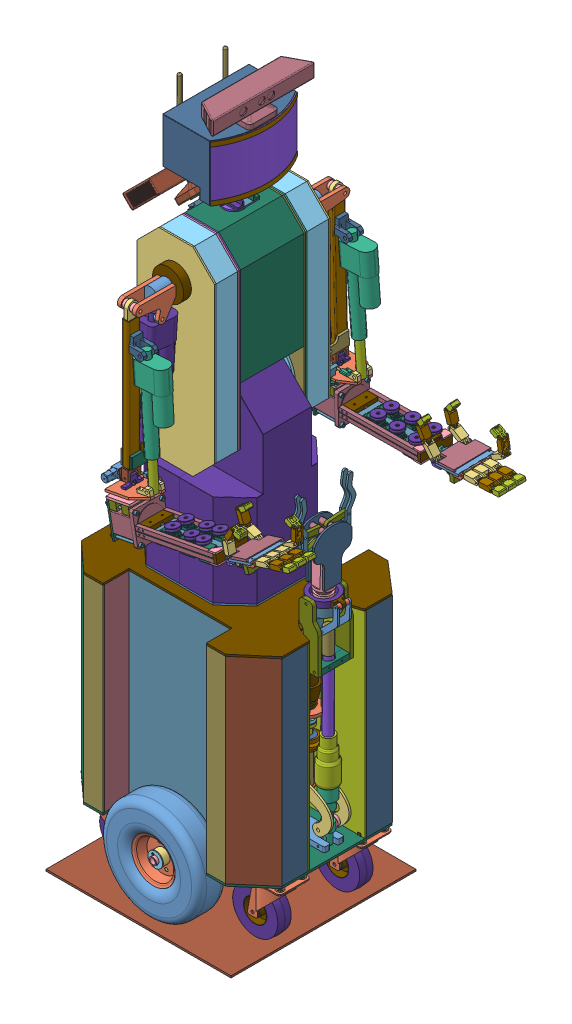
SolidWorks assembly sorbot, configuration По умолчанию. Lengths in mm. (continued)
Mates (geometry in assembly coordinates): (continued)
- Совпадение121: coincident anti-aligned: plane of bottom-2 through (-49.3372 51.9368 -286.1821) normal (0 1 0); plane of wall6-1 through (263.1742 51.9368 -58.2424) normal (0 -1 0)
- Совпадение122: coincident aligned: line of bottom-2 through (267.1742 51.9368 11.9714) axis (0 0 -1); line of wall6-1 through (267.1742 51.9368 11.8264) axis (0 0 -1)
- Параллельность26: parallel aligned: line of bottom-2 through (184.9009 51.9368 82.4522) axis (0.759435 0 -0.650583); line of wall7-1 through (184.8921 51.9368 82.4377) axis (0.759435 0 -0.650583)
- Совпадение127: coincident anti-aligned: plane of bottom-2 through (-49.3372 51.9368 -286.1821) normal (0 1 0); plane of wall7-1 through (263.5537 51.9368 9.7838) normal (0 -1 0)
- Совпадение131: coincident anti-aligned: line of bottom-2 through (267.1742 51.9368 11.9714) axis (0 0 -1); line of wall6-3 through (267.1742 51.9368 -286.3112) axis (0 0 1)
- Совпадение132: coincident anti-aligned: line of wall6-3 through (267.1742 51.9368 -216.2424) axis (0 1 0); line of wall2-2 through (267.1741 585.1505 -216.2424) axis (0 -1 0)
- Совпадение136: coincident aligned: line of bottom-2 through (132.9009 51.9368 12.4522) axis (0 0 1); line of wall8-1 through (132.9009 51.9368 78.4522) axis (0 0 1)
- Совпадение137: coincident aligned: line of bottom-2 through (132.9009 51.9368 82.4522) axis (1 0 0); line of wall8-1 through (132.9009 51.9368 82.4522) axis (1 0 0)
- Совпадение142: coincident anti-aligned: plane of bottom-2 through (-49.3372 51.9368 -286.1821) normal (0 1 0); plane of wall8-2 through (141.3107 51.9368 -178.9033) normal (0 -1 0)
- Совпадение143: coincident anti-aligned: plane of wall8-1 through (132.9009 637.4067 78.4522) normal (0 0 -1); plane of wall9-1 through (132.9009 655.1671 78.4522) normal (0 0 1)
- Совпадение144: coincident anti-aligned: plane of bottom-2 through (-49.3372 51.9368 -286.1821) normal (0 1 0); plane of wall9-1 through (132.9009 51.9368 78.4522) normal (0 -1 0)
- Совпадение145: coincident aligned: line of bottom-2 through (132.9009 51.9368 12.4522) axis (0 0 1); line of wall9-1 through (132.9009 51.9368 8.55) axis (0 0 1)
- Совпадение146: coincident aligned: line of bottom-2 through (39.4201 51.9368 12.4522) axis (1 0 0); line of wall10-1 through (-146.6756 51.9368 12.4522) axis (1 0 0)
- Совпадение147: coincident anti-aligned: plane of wall9-1 through (132.9009 655.1671 8.55) normal (-1 0 0); plane of wall10-1 through (132.9009 864.7556 8.4522) normal (1 0 0)
- Совпадение149: coincident anti-aligned: plane of bottom-2 through (-49.3372 51.9368 -286.1821) normal (0 1 0); plane of wall9-2 through (-150.6756 51.9368 78.5322) normal (0 -1 0)
- Совпадение157: coincident anti-aligned: line of wall3-1 through (107.1741 166.4368 -62.2424) axis (0 0 -1); line of wall4-1 through (107.1741 166.4368 -216.2424) axis (0 0 1)
- Совпадение161: coincident anti-aligned: line of wall2-2 through (21.1889 166.4368 -212.2424) axis (1 0 0); line of wall3-1 through (107.1741 166.4368 -212.2424) axis (-1 0 0)
- Совпадение162: coincident anti-aligned: line of wall2-1 through (107.1741 166.4368 -62.2424) axis (-1 0 0); line of wall3-1 through (26.1889 166.4368 -62.2424) axis (1 0 0)
- Совпадение170: coincident anti-aligned: plane of bottom-2 through (-49.3372 51.9368 -286.1821) normal (0 1 0); plane of wall7-v1-1 through (-149.98 51.9368 -93.7194) normal (0 -1 0)
- Параллельность29: parallel anti-aligned: line of bottom-2 through (-275.9596 51.9368 11.9714) axis (0.73854 0 0.67421); line of wall7-v1-1 through (-199.0366 51.9368 82.0998) axis (-0.73854 0 -0.67421)
- Совпадение174: coincident anti-aligned: line of wall7-v1-1 through (-275.9003 51.9368 11.9312) axis (0 1 0); line of wall11-1 through (-275.9003 585.1505 11.9312) axis (0 -1 0)
- Совпадение180: coincident anti-aligned: line of wall7-v1-2 through (-198.8179 51.9368 -356.1236) axis (0 1 0); line of wall8-5 through (-198.8179 585.1505 -356.1236) axis (0 -1 0)
- Совпадение181: coincident anti-aligned: plane of bottom-2 through (-49.3372 51.9368 -286.1821) normal (0 1 0); plane of wall8-5 through (-146.715 51.9368 -356.1236) normal (0 -1 0)
- Параллельность31: parallel aligned: line of bottom-2 through (-146.7539 51.9368 -356.1821) axis (-1 0 0); line of wall8-5 through (-146.715 51.9368 -356.1236) axis (-1 0 0)
- Совпадение182: coincident anti-aligned: plane of bottom-2 through (-49.3372 51.9368 -286.1821) normal (0 1 0); plane of wall9-3 through (-150.8245 51.9368 -282.1286) normal (0 -1 0)
- Совпадение184: coincident anti-aligned: plane of bottom-2 through (-49.3372 51.9368 -286.1821) normal (0 1 0); plane of wall10-v1-1 through (132.7521 51.9368 -286.1286) normal (0 -1 0)
- Совпадение187: coincident aligned: line of wall9-3 through (-146.8245 585.1505 -282.1286) axis (0 -1 0); line of wall10-v1-1 through (-146.8245 585.1505 -282.1286) axis (0 -1 0)
- Совпадение188: coincident anti-aligned: plane of bottom-2 through (-49.3372 51.9368 -286.1821) normal (0 1 0); plane of wall9-4 through (132.7521 51.9368 -282.1286) normal (0 -1 0)
- Совпадение189: coincident aligned: line of wall10-v1-1 through (132.7521 585.1505 -282.1286) axis (0 -1 0); line of wall9-4 through (132.7521 585.1505 -282.1286) axis (0 -1 0)
- Совпадение191: coincident anti-aligned: line of bottom-2 through (184.9009 51.9368 -356.1821) axis (-1 0 0); line of wall8-2 through (132.798 51.9368 -356.1821) axis (1 0 0)
- Совпадение201: coincident anti-aligned: plane of bottom-2 through (-49.3372 51.9368 -286.1821) normal (0 1 0); plane of wall7-3 through (183.3311 51.9368 -352.2595) normal (0 -1 0)
- Параллельность33: parallel aligned: line of bottom-2 through (267.1742 51.9368 -285.7013) axis (-0.759435 0 -0.650583); line of wall7-3 through (267.1973 51.9368 -285.6811) axis (-0.759435 0 -0.650583)
- Параллельность52: parallel anti-aligned: plane of gearmotor-3 through (-22.0648 623.1505 -128.1055) normal (-1 0 0); plane of turret-1/turret-p1-1 through (-22.0648 627.1934 -130.2473) normal (1 0 0)
- Концентричный93: concentric aligned: cylinder of gearmotor-3 through (-20.0648 629.1505 -136.9555) axis (0 -1 0) radius 7; cylinder of turret-1/turret-p1-1 through (-20.0648 627.1934 -136.9555) axis (0 -1 0) radius 7
- Концентричный110: concentric anti-aligned: cylinder of bolt1-2 through (172.9115 63.0264 3.3236) axis (0 -1 0) radius 5; cylinder of bolt1.nut-9 through (172.9115 51.9368 3.3236) axis (0 1 0) radius 5
- Концентричный111: concentric anti-aligned: cylinder of turret-1/turret-p1-1 through (-20.0648 603.2934 -136.9555) axis (0 1 0) radius 74; cylinder of turret.table-1 through (-20.0648 612.7934 -136.9555) axis (0 -1 0) radius 35
- Концентричный112: concentric aligned: cylinder of gearmotor-3 through (-20.0648 629.1505 -136.9555) axis (0 -1 0) radius 7; cylinder of turret.center-1 through (-20.0648 622.7934 -136.9555) axis (0 -1 0) radius 7
- Совпадение223: coincident anti-aligned: plane of turret-1/turret-p1-1 through (-20.0648 607.7934 -136.9555) normal (0 1 0); plane of ? through (-20.0648 607.7934 -136.9555) normal (0 -1 0)
- Совпадение230: coincident anti-aligned: plane of gearmotor.fixture.p2-3 through (10.2084 53.4933 -245.0001) normal (0 1 0); plane of wheel.axis.frame.fixture.p2-3 through (-51.698 53.4933 -213.5833) normal (0 -1 0)
- Совпадение236: coincident anti-aligned: plane of bottom-2 through (-49.3372 51.9368 -286.1821) normal (0 1 0); plane of wall-fixture-3-2 through (213.2226 51.9368 -31.5478) normal (0 -1 0)
- Совпадение242: coincident anti-aligned: plane of gearmotor-2 through (-40.8776 119.0545 -28.1692) normal (0 0 1); plane of gearmotor.fixture.p2.1-1 through (2.1309 53.4368 -28.1692) normal (0 0 -1)
- Совпадение246: coincident anti-aligned: plane of bottom-2 through (-49.3372 51.9368 -286.1821) normal (0 1 0); plane of wheel.axis.frame.fixture.p2-1 through (43.2929 51.9368 -36.1421) normal (0 -1 0)
- Совпадение248: coincident anti-aligned: plane of wheel.axis.frame-4 through (15.3082 32.4368 -66.3906) normal (0 -1 0); plane of wheel.axis.frame.fixture.p1-1 through (42.6901 32.4368 -36.0198) normal (0 1 0)
- Концентричный116: concentric aligned: circle of wheel.axis.frame.fixture.p1-1; circle of wheel.axis.frame.fixture.p2-1
- Совпадение252: coincident anti-aligned: plane of wall7-v1-1 through (-271.8817 585.1505 10.1837) normal (0 1 0); plane of cap-1 through (216.6954 585.1505 -83.7838) normal (0 -1 0)
- Совпадение253: coincident anti-aligned: plane of cap-1 through (216.6954 590.1505 -83.7838) normal (0 1 0); plane of turret-1/turret-p4-1 through (-19.4709 590.1505 -137.0226) normal (0 -1 0)
- Совпадение254: coincident anti-aligned: plane of turret-1/turret-p1-1 through (-20.0648 607.7934 -136.9555) normal (0 1 0); plane of turret.table-1 through (-20.0648 607.7934 -360.2969) normal (0 -1 0)
- Заблокировать30: lock: unknown of ?; unknown of ?
- Заблокировать31: lock: unknown of ?; unknown of ?
- Заблокировать32: lock: unknown of ?; unknown of ?
- Заблокировать33: lock: unknown of ?; unknown of ?
- Заблокировать34: lock: unknown of ?; unknown of ?
- Заблокировать35: lock: unknown of ?; unknown of ?
- Заблокировать36: lock: unknown of ?; unknown of ?
- Заблокировать37: lock: unknown of ?; unknown of ?
- Заблокировать38: lock: unknown of ?; unknown of ?
- Заблокировать39: lock: unknown of ?; unknown of ?
- Заблокировать40: lock: unknown of ?; unknown of ?
- Заблокировать41: lock: unknown of ?; unknown of ?
- Совпадение276: coincident anti-aligned: plane of bottom-2 through (-49.3372 51.9368 -286.1821) normal (0 1 0); plane of wall-fixture-3-3-1 through (-242.5877 51.9368 -17.2349) normal (0 -1 0)
- Совпадение277: coincident anti-aligned: plane of wall7-v1-1 through (-271.8817 -52.2153 10.1837) normal (0.67421 0 -0.73854); plane of wall-fixture-3-3-1 through (-269.5561 51.9368 12.3067) normal (-0.67421 0 0.73854)
- Заблокировать42: lock: unknown of ?; unknown of ?
- Заблокировать43: lock: unknown of ?; unknown of ?
- Заблокировать44: lock: unknown of ?; unknown of ?
- Заблокировать45: lock: unknown of ?; unknown of ?
- Заблокировать46: lock: unknown of ?; unknown of ?
- Заблокировать47: lock: unknown of ?; unknown of ?
- Заблокировать48: lock: unknown of ?; unknown of ?
- Заблокировать49: lock: unknown of ?; unknown of ?
- Заблокировать50: lock: unknown of ?; unknown of ?
- Заблокировать51: lock: unknown of ?; unknown of ?
- Заблокировать52: lock: unknown of ?; unknown of ?
- Заблокировать53: lock: unknown of ?; unknown of ?
- Совпадение282: coincident anti-aligned: plane of bottom-2 through (-49.3372 51.9368 -286.1821) normal (0 1 0); plane of bolt1.nut-1 through (-189.5596 51.9368 -278.9161) normal (0 -1 0)
- Заблокировать54: lock: unknown of ?; unknown of ?
- Заблокировать55: lock: unknown of ?; unknown of ?
- Заблокировать56: lock: unknown of ?; unknown of ?
- Заблокировать57: lock: unknown of ?; unknown of ?
- Заблокировать58: lock: unknown of ?; unknown of ?
- Заблокировать59: lock: unknown of ?; unknown of ?
- Заблокировать60: lock: unknown of ?; unknown of ?
- Заблокировать61: lock: unknown of ?; unknown of ?
- Заблокировать62: lock: unknown of ?; unknown of ?
- Заблокировать63: lock: unknown of ?; unknown of ?
- Заблокировать64: lock: unknown of ?; unknown of ?
- Заблокировать65: lock: unknown of ?; unknown of ?
- Совпадение287: coincident anti-aligned: plane of bottom-2 through (-49.3372 51.9368 -286.1821) normal (0 1 0); plane of bolt1.nut-9 through (180.9944 51.9368 3.3236) normal (0 -1 0)
- Заблокировать66: lock: unknown of ?; unknown of ?
- Заблокировать67: lock: unknown of ?; unknown of ?
- Заблокировать68: lock: unknown of ?; unknown of ?
- Заблокировать69: lock: unknown of ?; unknown of ?
- Заблокировать70: lock: unknown of ?; unknown of ?
- Заблокировать71: lock: unknown of ?; unknown of ?
- Заблокировать72: lock: unknown of ?; unknown of ?
- Заблокировать73: lock: unknown of ?; unknown of ?
- Заблокировать75: lock: unknown of ?; unknown of ?
- Заблокировать76: lock: unknown of ?; unknown of ?
- Заблокировать77: lock: unknown of ?; unknown of ?
- Совпадение290: coincident anti-aligned: plane of bottom-2 through (-49.3372 51.9368 -286.1821) normal (0 1 0); plane of bolt1.nut-13 through (164.6729 51.9368 -277.7529) normal (0 -1 0)
- Касательный1: tangent anti-aligned: cylinder of wheel-1/wheel.chamber-1 through (-6.6918 11.9368 97.7637) axis (0 0 -1) radius 135; plane of ground-1 through (232.7402 -123.0632 115.6816) normal (0 1 0)
- Концентричный125: concentric aligned: cylinder of body.center-1 through (-20.0648 982.0246 -136.9555) axis (0 -1 0) radius 11; cylinder of body_pivot_fixture-1 through (-20.0648 962.0246 -136.9555) axis (0 -1 0) radius 11
- Совпадение298: coincident anti-aligned: plane of turret.table-1 through (-20.0648 612.7934 -360.2969) normal (0 1 0); plane of body_tilt_drive_frame_p1-1 through (-111.0679 612.7934 -273.4555) normal (0 -1 0)
- Совпадение299: coincident: point of turret.table-1; unknown of body_tilt_drive_frame_p1-1
- Совпадение300: coincident: unknown of turret.table-1; unknown of body_tilt_drive_frame_p1-2
- Совпадение301: coincident anti-aligned: plane of turret.table-1 through (-20.0648 612.7934 -360.2969) normal (0 1 0); plane of body_tilt_drive_frame_p1-2 through (70.9352 612.7934 -0.4555) normal (0 -1 0)
- Совпадение315: coincident aligned: line of turret.table-1 through (-172.5648 612.7934 -54.9555) axis (0.73343 0 0.679765); line of body_tilt_drive_frame_p2-1 through (-172.514 612.7934 -54.9084) axis (0.73343 0 0.679765)
- Концентричный163: concentric aligned: cylinder of body_axis-1 through (-20.0648 1016.5246 -50.7475) axis (0 0 -1) radius 10.9; cylinder of body.frame.p1.fixture-2 through (-20.0648 1016.5246 -209.3595) axis (0 0 -1) radius 10.9
- Заблокировать91: lock: unknown of ?; unknown of ?
- Параллельность60: parallel aligned: cylinder of arm.actuator-1/arm.actuator.p1-1 through (-88.8064 993.1542 1.2558) axis (0 0 -1) radius 4.1; cylinder of arm.actuator.p2-1 through (-61.0144 1401.6056 11.2558) axis (0 0 -1) radius 4
- Концентричный165: concentric anti-aligned: cylinder of arm.actuator-1/arm.actuator.p1-1 through (-79.7097 1126.8451 -13.7442) axis (0.067885 0.997693 0) radius 10; cylinder of arm.actuator.p2-1 through (-60.4374 1410.086 -13.7442) axis (-0.067885 -0.997693 0) radius 10
- Концентричный454: concentric: cylinder of ? through (-88.5767 993.1387 1.2558) axis (0 0 -1) radius 4.1; cylinder of arm.lift.actuator.fixture.p2-1 through (-88.5767 993.1387 15.1693) axis (0 0 -1) radius 4
- Касательный32: tangent anti-aligned: cylinder of arm.actuator-1/arm.actuator.p1-1 through (-89.3495 985.1727 -13.7442) axis (0.067885 0.997693 0) radius 10; plane of arm.lift.actuator.fixture.p3-1 through (-88.5767 993.1387 -3.7442) normal (0 0 -1)
- Концентричный176: concentric aligned: cylinder of arm.actuator.p2-1 through (-61.0144 1401.6056 11.2558) axis (0 0 -1) radius 4; cylinder of shoulder.p4-1 through (-61.0144 1401.6056 -23.7442) axis (0 0 -1) radius 4
- Концентричный179: concentric aligned: cylinder of arm.actuator.p2-1 through (-61.0144 1401.6056 11.2558) axis (0 0 -1) radius 4; cylinder of shoulder.p4-2 through (-61.0144 1401.6056 0.2558) axis (0 0 -1) radius 4
- Концентричный183: concentric aligned: cylinder of arm.lift.actuator.fixture.p2-1 through (-88.5767 993.1387 15.1693) axis (0 0 -1) radius 4; cylinder of arm.lift.actuator.fixture.p3-1 through (-88.5767 993.1387 15.2558) axis (0 0 -1) radius 4
- Касательный11: tangent anti-aligned: cylinder of ? through (-60.4422 1410.0864 -13.7442) axis (-0.067324 -0.997731 0) radius 10; plane of ? through (-59.9468 1400.1462 -3.7442) normal (0 0 -1)
- Касательный12: tangent anti-aligned: cylinder of arm.actuator.p2-1 through (-60.4374 1410.086 -13.7442) axis (-0.067885 -0.997693 0) radius 10; plane of shoulder.p4-1 through (-59.9469 1400.1462 -23.7442) normal (0 0 1)
- Заблокировать105: lock: unknown of ?; unknown of ?
- Заблокировать106: lock: unknown of ?; unknown of ?
- Концентричный203: concentric anti-aligned: cylinder of arm.actuator-2/arm.actuator.p1-1 through (-12.7848 1153.0007 89.4303) axis (0 -0.997661 0.068351) radius 10; cylinder of arm.actuator.p2-2 through (-12.7848 967.3083 102.1523) axis (0 0.997661 -0.068351) radius 10
- Концентричный217: concentric anti-aligned: cylinder of arm.actuator100mm.p2-1 through (49.2564 930.6158 140.2746) axis (-0.061067 0.998134 0) radius 10; cylinder of arm.actuator100mm..p1-1 through (35.0693 1162.5008 140.2746) axis (0.061067 -0.998134 0) radius 10
- Параллельность77: parallel anti-aligned: cylinder of arm.actuator100mm..p1-1 through (29.8176 1248.3403 125.2746) axis (0 0 1) radius 4; cylinder of arm.actuator100mm.p2-1 through (48.7373 939.0999 165.2746) axis (0 0 -1) radius 4
- Заблокировать111: lock: unknown of ?; unknown of ?
- Заблокировать161: lock: unknown of ?; unknown of ?
- Совпадение447: coincident aligned: line of body_tilt_drive_frame_p6-2 through (128.9977 715.2934 -64.9448) axis (0 1 0); line of body_tilt_drive_frame_cap-1 through (128.9977 715.2934 -64.9448) axis (0 1 0)
- Концентричный281: concentric anti-aligned: cylinder of cap-hinge-1 through (95.4017 1325.4557 -46.5922) axis (0 -1 0) radius 2; cylinder of cap-hinge-p1-1 through (95.4017 1286.2182 -46.5922) axis (0 1 0) radius 2
- Совпадение460: coincident anti-aligned: plane of cap-hinge-1 through (75.4017 1315.4557 -52.4258) normal (0 -1 0); plane of cap-hinge-p1-1 through (75.4017 1315.4557 -51.5352) normal (0 1 0)
- Совпадение462: coincident anti-aligned: plane of arm.p1.m-1 through (-3.763 964.7884 152.9102) normal (1 0 0); plane of actuator.100.fixture-1 through (-3.763 1277.5198 127.4102) normal (-1 0 0)
- Совпадение463: coincident anti-aligned: line of arm.p1.m-1 through (-3.763 964.7884 127.4102) axis (0 1 0); line of actuator.100.fixture-1 through (-3.763 1277.5198 127.4102) axis (0 -1 0)
- Касательный17: tangent anti-aligned: cylinder of arm.actuator100mm..p1-1 through (29.329 1256.3254 140.2746) axis (0.061067 -0.998134 0) radius 10; plane of actuator.100.fixture-1 through (40.237 1209.783 150.2746) normal (0 0 -1)
- Концентричный291: concentric aligned: cylinder of arm.actuator100mm..p1-1 through (29.8176 1248.3403 125.2746) axis (0 0 1) radius 4; cylinder of actuator.100.fixture-1 through (29.8176 1248.3403 120.1602) axis (0 0 1) radius 4
- Заблокировать187: lock: unknown of ?; unknown of ?
- Заблокировать188: lock: unknown of ?; unknown of ?
- Заблокировать122: lock: unknown of ?; unknown of ?
- Концентричный297: concentric aligned: cylinder of arm.actuator.p2-2 through (12.2152 975.7884 101.5713) axis (-1 0 0) radius 4; cylinder of forearm.rotate.p12-1 through (-21.7679 975.7884 101.5713) axis (-1 0 0) radius 4
- Совпадение470: coincident: plane of ?; plane of ?
- Заблокировать196: lock: unknown of ?; unknown of ?
- Заблокировать207: lock: unknown of ?; unknown of ?
- Заблокировать208: lock: unknown of ?; unknown of ?
- Заблокировать216: lock: unknown of ?; unknown of ?
- Заблокировать217: lock: unknown of ?; unknown of ?
- Заблокировать218: lock: unknown of ?; unknown of ?
- Заблокировать219: lock: unknown of ?; unknown of ?
- Заблокировать220: lock: unknown of ?; unknown of ?
- Заблокировать221: lock: unknown of ?; unknown of ?
- Концентричный317: concentric anti-aligned: cylinder of HS-311 Hitec Standard Servo and Horn-1/HS-311-p2-1 through (119.3969 887.1533 157.9974) axis (-0.185706 0.982605 0) radius 4.064; cylinder of lower.arm.p9-1 through (118.2362 893.2946 157.9974) axis (0.185706 -0.982605 0) radius 12
- Совпадение569: coincident anti-aligned: plane of HS-311 Hitec Standard Servo and Horn-1/HS-311-p2-1 through (120.3857 893.7008 149.5983) normal (-0.185706 0.982605 0); plane of lower.arm.p9-1 through (118.2362 893.2946 157.9974) normal (0.185706 -0.982605 0)
- Заблокировать244: lock: unknown of ?; unknown of ?
- Концентричный318: concentric aligned: cylinder of HS-311 Hitec Standard Servo and Horn-3/HS-311-p2-1 through (119.3969 887.1533 122.4974) axis (-0.185706 0.982605 0) radius 4.064; cylinder of lower.arm.p9-2 through (119.1648 888.3816 122.4974) axis (-0.185706 0.982605 0) radius 4
- Концентричный319: concentric aligned: cylinder of HS-311 Hitec Standard Servo and Horn-2/HS-311-p2-1 through (173.4402 897.3672 119.9974) axis (-0.185706 0.982605 0) radius 4.064; cylinder of lower.arm.p9-5 through (173.2081 898.5954 119.9974) axis (-0.185706 0.982605 0) radius 4
- Концентричный320: concentric aligned: cylinder of HS-311 Hitec Standard Servo and Horn-4/HS-311-p2-1 through (207.1632 903.7406 117.4346) axis (-0.185706 0.982605 0) radius 4.064; cylinder of lower.arm.p9-6 through (206.9311 904.9689 117.4346) axis (-0.185706 0.982605 0) radius 4
- Концентричный321: concentric aligned: cylinder of HS-311 Hitec Standard Servo and Horn-5/HS-311-p2-1 through (173.4402 897.3672 160.9974) axis (-0.185706 0.982605 0) radius 4.064; cylinder of lower.arm.p9-4 through (173.2081 898.5954 160.9974) axis (-0.185706 0.982605 0) radius 4
- Концентричный322: concentric aligned: cylinder of HS-311 Hitec Standard Servo and Horn-6/HS-311-p2-1 through (207.1632 903.7406 163.1146) axis (-0.185706 0.982605 0) radius 4.064; cylinder of lower.arm.p9-3 through (206.9311 904.9689 163.1146) axis (-0.185706 0.982605 0) radius 4
- Совпадение570: coincident anti-aligned: plane of HS-311 Hitec Standard Servo and Horn-5/HS-311-p2-1 through (174.429 903.9147 152.5983) normal (-0.185706 0.982605 0); plane of lower.arm.p9-4 through (172.2795 903.5084 160.9974) normal (0.185706 -0.982605 0)
- Совпадение571: coincident anti-aligned: plane of HS-311 Hitec Standard Servo and Horn-6/HS-311-p2-1 through (203.8531 909.4756 171.5136) normal (-0.185706 0.982605 0); plane of lower.arm.p9-3 through (206.0025 909.8819 163.1146) normal (0.185706 -0.982605 0)
- Совпадение572: coincident anti-aligned: plane of HS-311 Hitec Standard Servo and Horn-3/HS-311-p2-1 through (120.3857 893.7008 114.0983) normal (-0.185706 0.982605 0); plane of lower.arm.p9-2 through (118.2362 893.2946 122.4974) normal (0.185706 -0.982605 0)
- Совпадение573: coincident anti-aligned: plane of HS-311 Hitec Standard Servo and Horn-2/HS-311-p2-1 through (174.429 903.9147 111.5983) normal (-0.185706 0.982605 0); plane of lower.arm.p9-5 through (172.2795 903.5084 119.9974) normal (0.185706 -0.982605 0)
- Совпадение574: coincident anti-aligned: plane of HS-311 Hitec Standard Servo and Horn-4/HS-311-p2-1 through (203.8531 909.4756 125.8336) normal (-0.185706 0.982605 0); plane of lower.arm.p9-6 through (206.0025 909.8819 117.4346) normal (0.185706 -0.982605 0)
- Заблокировать245: lock: unknown of ?; unknown of ?
- Заблокировать246: lock: unknown of ?; unknown of ?
- Заблокировать247: lock: unknown of ?; unknown of ?
- Заблокировать248: lock: unknown of ?; unknown of ?
- Заблокировать249: lock: unknown of ?; unknown of ?
- Заблокировать250: lock: unknown of ?; unknown of ?
- Совпадение582: coincident anti-aligned: plane of palm.p1-3 through (364.9952 940.9838 91.5947) normal (0.311571 -0.950223 0); plane of palm.p3-1 through (346.841 935.0312 91.3484) normal (-0.311571 0.950223 0)
- Совпадение583: coincident anti-aligned: plane of palm.p1-3 through (361.9011 946.2836 191.5864) normal (0.950144 0.311545 0.012888); plane of palm.p3-1 through (362.0352 950.0109 91.5947) normal (-0.950144 -0.311545 -0.012888)
- Совпадение584: coincident aligned: plane of palm.p1-3 through (290.6402 922.9177 190.6197) normal (-0.012247 -0.004016 0.999917); plane of palm.p3-1 through (369.3773 952.4183 191.7026) normal (-0.012247 -0.004016 0.999917)
- Заблокировать261: lock: unknown of ?; unknown of ?
- Заблокировать262: lock: unknown of ?; unknown of ?
- Заблокировать265: lock: unknown of ?; unknown of ?
- Заблокировать266: lock: unknown of ?; unknown of ?
- Концентричный332: concentric aligned: cylinder of palm.p3-1 through (367.5649 947.6145 91.6528) axis (-0.012247 -0.004016 0.999917) radius 1.5; cylinder of finger.p1-1 through (366.6096 947.3013 169.6463) axis (-0.012247 -0.004016 0.999917) radius 1.5
- Концентричный333: concentric anti-aligned: cylinder of finger.p1-1 through (366.6096 947.3013 169.6463) axis (-0.012247 -0.004016 0.999917) radius 1.5; cylinder of finger.spring-1 through (366.5011 947.2657 178.5056) axis (0.012247 0.004016 -0.999917) radius 1.9307
- Касательный23: tangent anti-aligned: plane of finger.p1-1 through (351.8589 937.2027 182.1761) normal (0.012247 0.004016 -0.999917); cylinder of finger.spring-1 through (357.2133 941.7472 181.9199) axis (0.950144 0.311545 0.012888) radius 0.34
- Параллельность161: parallel aligned: plane of finger.p1-1 through (363.4168 940.9924 169.5819) normal (-0.950144 -0.311545 -0.012888); plane of finger.spring-1 through (357.2133 941.7472 181.9199) normal (-0.950144 -0.311545 -0.012888)
- Концентричный334: concentric aligned: cylinder of palm.p3-1 through (367.5649 947.6145 91.6528) axis (-0.012247 -0.004016 0.999917) radius 1.5; cylinder of palm.fixture.p13-1 through (367.5656 947.6147 91.5963) axis (-0.012247 -0.004016 0.999917) radius 1.5
- Совпадение627: coincident anti-aligned: plane of palm.p3-1 through (362.243 935.8718 186.5483) normal (0.012247 0.004016 -0.999917); plane of finger.p1-1 through (357.4065 939.0217 186.5017) normal (-0.012247 -0.004016 0.999917)
- Параллельность160: parallel aligned: plane of palm.p1-3 through (363.1257 946.6851 91.5947) normal (-0.311571 0.950223 0); plane of finger.p1-1 through (406.9341 967.89 190.7246) normal (-0.311571 0.950223 0)
- Концентричный339: concentric aligned: cylinder of palm.fixture.p13-1 through (367.5656 947.6147 91.5963) axis (-0.012247 -0.004016 0.999917) radius 1.5; cylinder of finger.p1-2 through (367.5465 947.6085 93.1527) axis (-0.012247 -0.004016 0.999917) radius 1.5
- Концентричный342: concentric aligned: cylinder of palm.fixture.p13-1 through (367.5656 947.6147 91.5963) axis (-0.012247 -0.004016 0.999917) radius 1.5; cylinder of finger.p1-3 through (366.9219 947.4037 144.1484) axis (-0.012247 -0.004016 0.999917) radius 1.5
- Параллельность165: parallel aligned: plane of palm.p1-3 through (363.1257 946.6851 91.5947) normal (-0.311571 0.950223 0); plane of finger.p1-3 through (407.2464 967.9924 165.2267) normal (-0.311571 0.950223 0)
- Совпадение637: coincident anti-aligned: plane of palm.p1-3 through (364.9952 940.9838 91.5947) normal (0.311571 -0.950223 0); plane of palm.p3.m-1 through (323.3155 927.3173 191.0376) normal (-0.311571 0.950223 0)
- Совпадение638: coincident aligned: plane of palm.p1-3 through (290.6402 922.9177 190.6197) normal (-0.012247 -0.004016 0.999917); plane of palm.p3.m-1 through (290.9518 925.1246 190.6324) normal (-0.012247 -0.004016 0.999917)
- Совпадение640: coincident anti-aligned: plane of palm.p3.m-1 through (299.2015 928.9006 190.7486) normal (0.950144 0.311545 0.012888); plane of palm.p1-3 through (300.4356 926.1295 166.7506) normal (-0.950144 -0.311545 -0.012888)
- Совпадение641: coincident anti-aligned: plane of palm.p3-1 through (363.3452 936.2333 96.5558) normal (-0.012247 -0.004016 0.999917); plane of finger.p1-2 through (360.8495 937.3933 96.5299) normal (0.012247 0.004016 -0.999917)
- Концентричный345: concentric aligned: cylinder of palm.fixture.p13-1 through (367.5656 947.6147 91.5963) axis (-0.012247 -0.004016 0.999917) radius 1.5; cylinder of finger.p1-4 through (367.2342 947.5061 118.6505) axis (-0.012247 -0.004016 0.999917) radius 1.5
- Параллельность167: parallel aligned: plane of palm.p1-3 through (363.1257 946.6851 91.5947) normal (-0.311571 0.950223 0); plane of finger.p1-4 through (407.5587 968.0948 139.7288) normal (-0.311571 0.950223 0)
- Совпадение645: coincident anti-aligned: plane of palm.p1-3 through (364.9952 940.9838 91.5947) normal (0.311571 -0.950223 0); plane of palm.p3.m-2 through (324.2768 927.6326 112.5441) normal (-0.311571 0.950223 0)
- Совпадение646: coincident aligned: plane of palm.p1-3 through (291.8649 923.3193 90.628) normal (0.012247 0.004016 -0.999917); plane of palm.p3.m-2 through (292.1765 925.5262 90.6407) normal (0.012247 0.004016 -0.999917)
- Совпадение647: coincident anti-aligned: plane of palm.p3.m-2 through (300.1629 929.2158 112.2551) normal (0.950144 0.311545 0.012888); plane of palm.p1-3 through (301.0725 926.3383 114.7549) normal (-0.950144 -0.311545 -0.012888)
- Заблокировать267: lock: unknown of ?; unknown of ?
- Концентричный348: concentric aligned: cylinder of palm.p3.m-1 through (296.5509 922.5164 190.6905) axis (0.012247 0.004016 -0.999917) radius 1.5; cylinder of finger.p1-5 through (296.557 922.5184 190.1906) axis (0.012247 0.004016 -0.999917) radius 1.5
- Совпадение648: coincident anti-aligned: plane of palm.p3.m-1 through (289.0079 911.8586 186.555) normal (0.012247 0.004016 -0.999917); plane of finger.p1-5 through (294.0033 910.6326 186.6113) normal (-0.012247 -0.004016 0.999917)
- Концентричный351: concentric aligned: cylinder of finger.p1-6 through (297.5172 922.8332 111.7971) axis (0.012247 0.004016 -0.999917) radius 1.5; cylinder of palm.p3.m-2 through (297.5123 922.8316 112.197) axis (0.012247 0.004016 -0.999917) radius 1.5
- Концентричный352: concentric aligned: cylinder of finger.p1-1 through (405.2463 959.4437 170.1683) axis (-0.012247 -0.004016 0.999917) radius 1.5; cylinder of finger.p2-7 through (405.2463 959.4437 170.1683) axis (-0.012247 -0.004016 0.999917) radius 1.5
- Совпадение652: coincident anti-aligned: plane of finger.p1-1 through (399.3202 952.7649 186.5702) normal (0.012247 0.004016 -0.999917); plane of finger.p2-7 through (396.174 952.0257 186.5287) normal (-0.012247 -0.004016 0.999917)
- Концентричный354: concentric: cylinder of finger.p3-1 through (466.5916 802.6812 273.0909) axis (-0.001318 0.191299 0.981531) radius 1.5; cylinder of ? through (466.5917 802.6596 272.9801) axis (-0.001318 0.191299 0.981531) radius 1.5
- Совпадение653: coincident: plane of ? through (235.2448 521.1837 179.8569) normal (0.004463 0.000114 0.99999); plane of ? through (237.0318 518.7761 179.8492) normal (-0.004463 -0.000114 -0.99999)
- Концентричный355: concentric aligned: cylinder of finger.p1-3 through (405.5586 959.5461 144.6704) axis (-0.012247 -0.004016 0.999917) radius 1.5; cylinder of finger.p2-8 through (405.5586 959.5461 144.6704) axis (-0.012247 -0.004016 0.999917) radius 1.5
- Совпадение654: coincident anti-aligned: plane of finger.p1-3 through (399.6325 952.8673 161.0724) normal (0.012247 0.004016 -0.999917); plane of finger.p2-8 through (396.6473 951.938 161.0321) normal (-0.012247 -0.004016 0.999917)
- Концентричный356: concentric aligned: cylinder of finger.p1-4 through (405.8709 959.6485 119.1725) axis (-0.012247 -0.004016 0.999917) radius 1.5; cylinder of finger.p2-9 through (405.8709 959.6485 119.1725) axis (-0.012247 -0.004016 0.999917) radius 1.5
- Совпадение655: coincident anti-aligned: plane of finger.p1-4 through (399.9448 952.9697 135.5745) normal (0.012247 0.004016 -0.999917); plane of finger.p2-9 through (396.9974 951.997 135.5345) normal (-0.012247 -0.004016 0.999917)
- Концентричный357: concentric aligned: cylinder of finger.p1-2 through (401.9154 969.0333 93.6596) axis (-0.012247 -0.004016 0.999917) radius 1.5; cylinder of finger.p2-10 through (401.9154 969.0333 93.6596) axis (-0.012247 -0.004016 0.999917) radius 1.5
- Совпадение656: coincident anti-aligned: plane of finger.p1-2 through (397.826 961.1324 110.0792) normal (0.012247 0.004016 -0.999917); plane of finger.p2-10 through (406.346 958.4178 110.1726) normal (-0.012247 -0.004016 0.999917)
- Концентричный358: concentric aligned: cylinder of finger.p3-2 through (401.4238 1008.0295 93.9231) axis (-0.012247 -0.004016 0.999917) radius 1.5; cylinder of finger.p2-10 through (401.4252 1008.0299 93.8102) axis (-0.012247 -0.004016 0.999917) radius 1.5
- Совпадение657: coincident anti-aligned: plane of ? through (412.7357 1007.5295 110.4481) normal (-0.012247 -0.004016 0.999917); plane of finger.p2-10 through (405.8167 1000.5207 110.3352) normal (0.012247 0.004016 -0.999917)
- Концентричный359: concentric aligned: cylinder of finger.p1-5 through (287.6988 962.0409 190.2408) axis (0.012247 0.004016 -0.999917) radius 1.5; cylinder of finger.p2-11 through (287.6988 962.0409 190.2408) axis (0.012247 0.004016 -0.999917) radius 1.5
- Совпадение658: coincident anti-aligned: plane of finger.p1-5 through (284.8951 953.7891 186.173) normal (0.012247 0.004016 -0.999917); plane of finger.p2-11 through (278.3955 955.3292 186.0996) normal (-0.012247 -0.004016 0.999917)
- Концентричный360: concentric aligned: cylinder of finger.p3-5 through (307.9454 995.3702 190.7355) axis (0.012247 0.004016 -0.999917) radius 1.5; cylinder of finger.p2-11 through (307.9467 995.3707 190.6226) axis (0.012247 0.004016 -0.999917) radius 1.5
- Совпадение659: coincident anti-aligned: plane of finger.p3-5 through (298.337 1001.6675 186.5299) normal (-0.012247 -0.004016 0.999917); plane of finger.p2-11 through (300.2563 991.3138 186.5118) normal (0.012247 0.004016 -0.999917)
- Концентричный362: concentric aligned: cylinder of ? through (259.3107 936.2716 111.3831) axis (0.012247 0.004016 -0.999917) radius 1.5; cylinder of finger.p2-12 through (259.3107 936.2716 111.3831) axis (0.012247 0.004016 -0.999917) radius 1.5
- Совпадение661: coincident anti-aligned: plane of ? through (264.8581 929.4858 107.4234) normal (0.012247 0.004016 -0.999917); plane of ? through (259.1122 924.7688 107.3341) normal (-0.012247 -0.004016 0.999917)
- Концентричный363: concentric aligned: cylinder of finger.p3-6 through (195.7839 707.1121 106.7239) axis (-0.004463 -0.000114 -0.99999) radius 1.5; cylinder of ? through (195.7834 707.1121 106.6111) axis (-0.004463 -0.000114 -0.99999) radius 1.5
- Совпадение662: coincident: plane of ? through (190.3026 717.2558 102.6343) normal (0.004463 0.000114 0.99999); plane of ? through (187.0589 706.2794 102.6501) normal (-0.004463 -0.000114 -0.99999)
- Совпадение664: coincident anti-aligned: plane of palm.p3-1 through (373.957 939.7128 161.2051) normal (0.012247 0.004016 -0.999917); plane of finger.p1-3 through (357.7188 939.1241 161.0039) normal (-0.012247 -0.004016 0.999917)
- Совпадение665: coincident anti-aligned: plane of palm.p3-1 through (374.2693 939.8152 135.7072) normal (0.012247 0.004016 -0.999917); plane of finger.p1-4 through (358.0311 939.2265 135.506) normal (-0.012247 -0.004016 0.999917)
- Совпадение666: coincident anti-aligned: plane of palm.p1-3 through (363.1257 946.6851 91.5947) normal (-0.311571 0.950223 0); plane of palm.p5-1 through (330.6828 936.0474 170.4076) normal (0.311571 -0.950223 0)
- Совпадение667: coincident anti-aligned: plane of palm.p1-3 through (363.1257 946.6851 91.5947) normal (-0.311571 0.950223 0); plane of palm.p6-1 through (301.0674 926.3367 156.6492) normal (0.311571 -0.950223 0)
- Совпадение668: coincident anti-aligned: plane of palm.p1-3 through (363.1257 946.6851 91.5947) normal (-0.311571 0.950223 0); plane of palm.p5-2 through (331.3758 936.2746 112.4456) normal (0.311571 -0.950223 0)
- Совпадение669: coincident anti-aligned: plane of palm.p1-3 through (363.1257 946.6851 91.5947) normal (-0.311571 0.950223 0); plane of palm.p6-2 through (301.386 926.4412 124.555) normal (0.311571 -0.950223 0)
- Заблокировать268: lock: unknown of ?; unknown of ?
- Совпадение692: coincident anti-aligned: plane of arm.p1.m-1 through (-3.763 964.7884 152.9102) normal (1 0 0); plane of forearm.rotate.p12-m-1 through (-3.763 985.2277 154.0338) normal (-1 0 0)
- Параллельность178: parallel aligned: plane of forearm.rotate.p12-m-1 through (-3.763 964.7884 154.0338) normal (0 0 1); plane of arm.p1.m-1 through (-18.263 964.7884 156.4102) normal (0 0 1)
- Заблокировать282: lock: unknown of ?; unknown of ?
- Концентричный381: concentric aligned: cylinder of finger.p3-3 through (442.6662 971.5314 145.2986) axis (-0.012247 -0.004016 0.999917) radius 1.5; cylinder of finger.p2-8 through (442.6677 971.5319 145.173) axis (-0.012247 -0.004016 0.999917) radius 1.5
- Концентричный382: concentric aligned: cylinder of finger.p3-4 through (442.9206 971.8199 119.5969) axis (-0.012247 -0.004016 0.999917) radius 1.5; cylinder of finger.p2-9 through (442.9196 971.8196 119.6752) axis (-0.012247 -0.004016 0.999917) radius 1.5
- Заблокировать287: lock: unknown of ?; unknown of ?
- Заблокировать288: lock: unknown of ?; unknown of ?
- Заблокировать290: lock: unknown of ?; unknown of ?
- Заблокировать291: lock: unknown of ?; unknown of ?
- Заблокировать293: lock: unknown of ?; unknown of ?
- Заблокировать294: lock: unknown of ?; unknown of ?
- Заблокировать295: lock: unknown of ?; unknown of ?
- Заблокировать296: lock: unknown of ?; unknown of ?
- Заблокировать297: lock: unknown of ?; unknown of ?
- Заблокировать298: lock: unknown of ?; unknown of ?
- Заблокировать299: lock: unknown of ?; unknown of ?
- Заблокировать301: lock: unknown of ?; unknown of ?
- Заблокировать302: lock: unknown of ?; unknown of ?
- Заблокировать304: lock: unknown of ?; unknown of ?
- Заблокировать305: lock: unknown of ?; unknown of ?
- Заблокировать306: lock: unknown of ?; unknown of ?
- Заблокировать307: lock: unknown of ?; unknown of ?
- Заблокировать308: lock: unknown of ?; unknown of ?
- Заблокировать309: lock: unknown of ?; unknown of ?
- Заблокировать310: lock: unknown of ?; unknown of ?
- Заблокировать311: lock: unknown of ?; unknown of ?
- Заблокировать319: lock: unknown of ?; unknown of ?
- Концентричный386: concentric aligned: cylinder of body.frame.p1-3 through (-12.4559 1335.4922 -50.7442) axis (0 0 1) radius 43; cylinder of arm.fixture.cap-1 through (-12.4559 1335.4922 -73.2442) axis (0 0 1) radius 45
- Заблокировать330: lock: unknown of ?; unknown of ?
- Заблокировать336: lock: unknown of ?; unknown of ?
- Заблокировать337: lock: unknown of ?; unknown of ?
- Заблокировать344: lock: unknown of body_tilt_drive_frame_cap-1; unknown of ?
- Заблокировать351: lock: unknown of turret.table.cap-1; unknown of body_tilt_drive_frame_cap-1
- Совпадение740: coincident anti-aligned: plane of shoulder.bearing.housing-2 through (-12.4903 1335.516 -46.7442) normal (0 0 1); plane of body.frame.p4.right-1 through (-117.4903 1436.2936 -46.7442) normal (0 0 -1)
- Концентричный404: concentric aligned: cylinder of shoulder.bearing.housing-1 through (-12.7629 1335.3853 40.2558) axis (0 0 -1) radius 15.5; cylinder of shoulder.axis-1 through (-12.7629 1335.3853 44.2558) axis (0 0 -1) radius 15
- Совпадение742: coincident: plane of ?; plane of ?
- Заблокировать361: lock: unknown of ?; unknown of ?
- Заблокировать362: lock: unknown of ?; unknown of ?
- Совпадение745: coincident anti-aligned: plane of body.frame.p5-1 through (92.4017 957.5916 592.5032) normal (1 0 0); plane of cap-hinge-1 through (92.4017 1325.4557 -46.5922) normal (-1 0 0)
- Совпадение746: coincident anti-aligned: plane of body.frame.p5-1 through (92.4017 957.5916 592.5032) normal (1 0 0); plane of cap-hinge-p1-2 through (92.4017 1182.6154 -46.8053) normal (-1 0 0)
- Концентричный405: concentric anti-aligned: cylinder of cap-hinge-2 through (95.4017 1143.4534 -46.8053) axis (0 1 0) radius 2; cylinder of cap-hinge-p1-2 through (95.4017 1182.6154 -46.8053) axis (0 -1 0) radius 2
- Совпадение747: coincident anti-aligned: plane of cap-hinge-2 through (75.4017 1173.4534 -40.9717) normal (0 -1 0); plane of cap-hinge-p1-2 through (75.4017 1173.4534 -41.8622) normal (0 1 0)
- Заблокировать363: lock: unknown of ?; unknown of ?
- Заблокировать364: lock: cylinder of ?; plane of ?
- Касательный31: tangent anti-aligned: cylinder of arm.actuator.p2-2 through (-12.7848 967.3083 102.1523) axis (0 0.997661 -0.068351) radius 10; plane of forearm.rotate.p12-1 through (-22.7848 999.7884 125.248) normal (1 0 0)
- Параллельность188: parallel anti-aligned: cylinder of arm.actuator-2/arm.actuator.p1-1 through (-27.7848 1286.6873 80.2712) axis (1 0 0) radius 4.1; cylinder of arm.actuator.p2-2 through (12.2152 975.7884 101.5713) axis (-1 0 0) radius 4
- Заблокировать368: lock: unknown of ?; unknown of ?
- Заблокировать369: lock: unknown of ?; unknown of ?
- Совпадение765: coincident anti-aligned: plane of arm.p1.m-1 through (-18.263 964.7884 125.9102) normal (0 0 1); plane of shoulder.lever-1 through (-17.763 1335.3853 125.9102) normal (0 0 -1)
- Концентричный406: concentric anti-aligned: cylinder of ? through (-27.7629 1335.3853 140.1602) axis (-1 0 0) radius 4; cylinder of shoulder.lever-1 through (-17.763 1335.3853 140.1602) axis (1 0 0) radius 4
- Концентричный408: concentric aligned: cylinder of arm.lift2.actuator.fixture.p1-1 through (-17.763 1335.3853 140.1602) axis (-1 0 0) radius 4; cylinder of ? through (-27.7629 1335.3853 140.1602) axis (-1 0 0) radius 4
- Совпадение757: coincident anti-aligned: plane of shoulder.lever-1 through (-17.763 1335.3853 140.1608) normal (-1 0 0); plane of ? through (-17.763 1335.3853 140.1602) normal (1 0 0)
- Концентричный409: concentric anti-aligned: cylinder of arm.actuator-2/arm.actuator.p1-1 through (-27.7848 1286.6873 80.2712) axis (1 0 0) radius 4.1; cylinder of ? through (-27.7629 1286.6873 80.2712) axis (-1 0 0) radius 4
- Совпадение759: coincident anti-aligned: plane of ? through (-27.7629 1335.3734 139.2441) normal (1 0 0); plane of arm.lift2.actuator.fixture.p1.m1-1 through (-27.7629 1286.6873 80.2712) normal (-1 0 0)
- Концентричный411: concentric anti-aligned: cylinder of arm.actuator-2/arm.actuator.p1-1 through (-27.7848 1286.6873 80.2712) axis (1 0 0) radius 4.1; cylinder of ? through (-22.7629 1286.6873 80.2712) axis (-1 0 0) radius 4
- Совпадение760: coincident anti-aligned: plane of ? through (2.2371 1356.1502 -67.7442) normal (1 0 0); plane of arm.fixture-3 through (2.2371 1335.3734 139.2441) normal (-1 0 0)
- Концентричный412: concentric anti-aligned: cylinder of shoulder.lever-1 through (-17.763 1335.3853 140.1602) axis (1 0 0) radius 4; cylinder of ? through (12.2371 1335.3853 140.1602) axis (-1 0 0) radius 4
- Концентричный413: concentric aligned: cylinder of ? through (12.2371 1335.3853 140.1602) axis (-1 0 0) radius 4; cylinder of arm.lift2.actuator.fixture.p1-3 through (2.2371 1335.3853 140.1602) axis (-1 0 0) radius 4
- Совпадение761: coincident anti-aligned: plane of ? through (2.2371 1335.3734 139.2441) normal (-1 0 0); plane of ? through (2.2371 1335.3853 140.1602) normal (1 0 0)
- Концентричный414: concentric anti-aligned: cylinder of arm.actuator-2/arm.actuator.p1-1 through (-27.7848 1286.6873 80.2712) axis (1 0 0) radius 4.1; cylinder of arm.lift2.actuator.fixture.p1.m1-2 through (2.2371 1286.6873 80.2712) axis (-1 0 0) radius 4
- Совпадение762: coincident anti-aligned: plane of ? through (2.2371 1335.3734 139.2441) normal (-1 0 0); plane of ? through (2.2371 1286.6873 80.2712) normal (1 0 0)
- Концентричный416: concentric anti-aligned: cylinder of arm.actuator-2/arm.actuator.p1-1 through (-27.7848 1286.6873 80.2712) axis (1 0 0) radius 4.1; cylinder of ? through (12.2371 1286.6873 80.2712) axis (-1 0 0) radius 4
- Заблокировать370: lock: unknown of ?; unknown of ?
- Концентричный420: concentric aligned: cylinder of body.center-1 through (-20.0648 982.0246 -136.9555) axis (0 -1 0) radius 11; cylinder of body_pivot-2 through (-20.0648 982.0246 -136.9555) axis (0 -1 0) radius 11
- Заблокировать371: lock: unknown of body.center-1; unknown of body_pivot_fixture-1
- Совпадение768: coincident anti-aligned: plane of body_pivot_fixture-1 through (-20.0648 972.0246 -136.9555) normal (0 1 0); plane of ? through (-63.8424 972.0246 -151.4602) normal (0 -1 0)
- Заблокировать372: lock: unknown of ?; unknown of ?
- Концентричный421: concentric anti-aligned: cylinder of body_axis-1 through (-20.0648 1016.5246 -50.7475) axis (0 0 -1) radius 10.9; cylinder of body.tilt.axis.frame-2 through (-20.0648 1016.5246 -110.5942) axis (0 0 1) radius 11
- Совпадение776: coincident anti-aligned: plane of ? through (-63.8424 982.0246 -151.4602) normal (0 1 0); plane of ? through (1.9352 982.0246 -116.0942) normal (0 -1 0)
- Концентричный422: concentric aligned: cylinder of body_axis-1 through (-20.0648 1016.5246 -50.7475) axis (0 0 -1) radius 10.9; cylinder of body.tilt.axis.frame-3 through (-20.0648 1016.5246 -163.4875) axis (0 0 -1) radius 11
- Совпадение779: coincident anti-aligned: plane of ? through (-63.8424 982.0246 -151.4602) normal (0 1 0); plane of ? through (1.9352 982.0246 -157.9875) normal (0 -1 0)
- Совпадение783: coincident aligned: plane of body_tilt_drive_frame_cap-1 through (-173.1373 715.2934 -206.9448) normal (0 0 -1); plane of body_tilt_drive_frame_p6-3 through (-171.1373 1083.0403 -206.9448) normal (0 0 -1)
- Концентричный430: concentric anti-aligned: cylinder of tilt.thread.rod-1 through (-119.3768 948.5591 -141.6211) axis (0 -1 0) radius 8; cylinder of tilt.thread.rod.fixture.2-1 through (-119.3768 794.5591 -141.6211) axis (0 1 0) radius 8
- Совпадение797: coincident anti-aligned: plane of tilt.thread.rod-1 through (-119.3768 794.5591 -141.6211) normal (0 -1 0); plane of tilt.thread.rod.fixture.2-1 through (-119.3768 794.5591 -141.6211) normal (0 1 0)
- Концентричный431: concentric: cylinder of ? through (-118.5699 947.5591 -137.5376) axis (0 -1 0) radius 8; cylinder of tilit.thread.rod.bearing.fixture-1 through (-118.5701 937.0246 -137.4966) axis (0 -1 0) radius 6.5
- Совпадение799: coincident anti-aligned: plane of tilit.thread.rod.bearing.fixture-1 through (-20.0648 937.0246 -136.9555) normal (0 1 0); plane of tilit.thread.bearing-1 through (-119.3768 937.0246 -141.6211) normal (0 -1 0)
- Концентричный432: concentric anti-aligned: cylinder of tilt.thread.rod-1 through (-119.3768 928.5591 -141.6211) axis (0 1 0) radius 6; cylinder of ? through (-119.3768 945.0246 -141.6211) axis (0 -1 0) radius 6
- Совпадение800: coincident anti-aligned: plane of tilit.thread.rod.bearing.fixture-1 through (-20.0648 937.0246 -136.9555) normal (0 1 0); plane of tilit.thread.rod.bearing.housing-1 through (-119.3768 937.0246 -141.6211) normal (0 -1 0)
- Концентричный433: concentric aligned: cylinder of ? through (-119.3768 945.0246 -141.6211) axis (0 -1 0) radius 14; cylinder of ? through (-119.3768 945.0246 -141.6211) axis (0 -1 0) radius 14
- Концентричный434: concentric anti-aligned: cylinder of body_axis-1 through (-20.0648 1016.5246 -50.7475) axis (0 0 -1) radius 10.9; cylinder of body_tilt_axis_clamp-1 through (-20.0648 1016.5246 -155.4875) axis (0 0 1) radius 11
